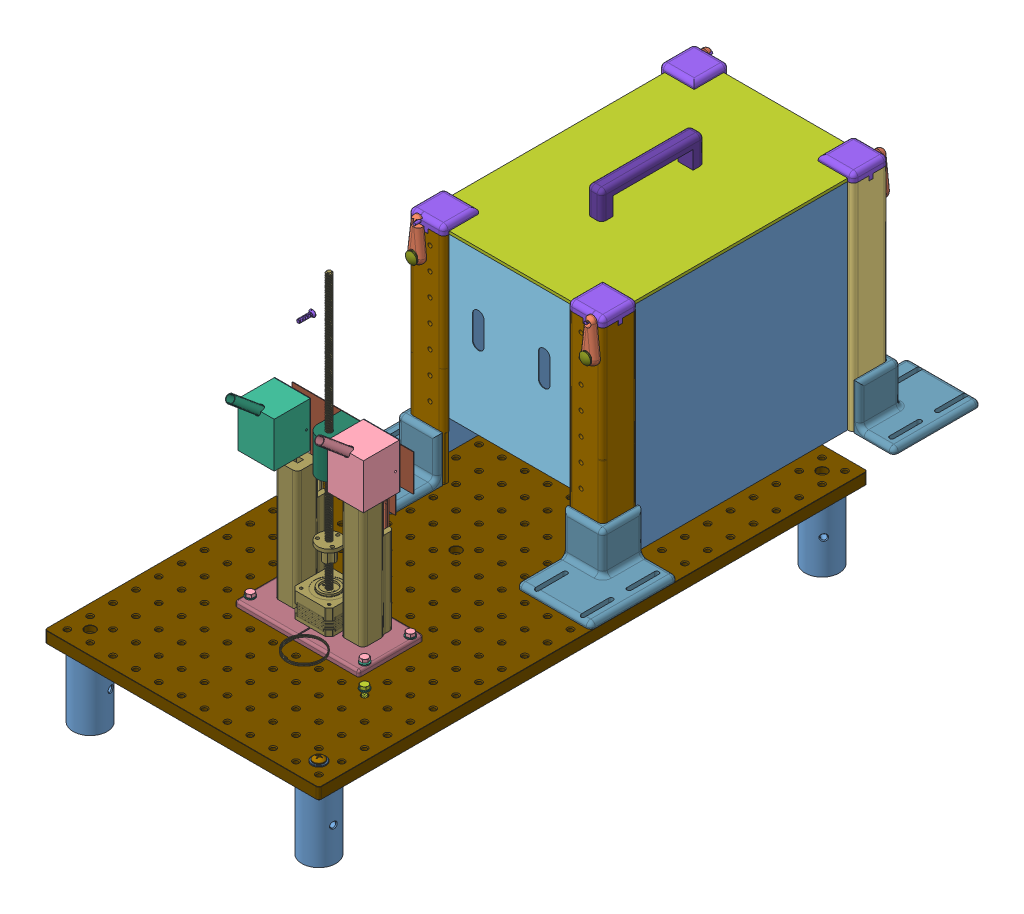
SolidWorks assembly Cage_model, configuration Default. Lengths in mm.
Overall size (306.09 428.48 734.93).
48 component instances, 32 part files, 99 mates.
Components (placement in the parent):
- Cage_acryllic_main-1: Cage_acryllic_main [Default] at (116.4275 -22.4186 -670.5141) size (203.2 239 304.17)
- Locking Mechanism^Cage_model-1: Locking Mechanism^Cage_model [Default] at (119.1314 -13.6836 -620.5993) x (0.989545 0 -0.144222) z (0.144222 0 0.989545) size (209.18 47.14 36.28) (virtual)
- Rear Legs^Cage_model-1: Rear Legs^Cage_model [Default] at (116.4275 -20.4186 -670.5141) x (0 0 -1) z (1 0 0) size (39.08 239 215.9) (virtual)
- Copy of Copy of Tube_Housing^Cage_model-1: Copy of Copy of Tube_Housing^Cage_model [Default] at (-6024.2431 5876.1322 -191.2968) size (40 77.55 71.62) (virtual)
- Stainless_steel_faceplate^Cage_model-1: Stainless_steel_faceplate^Cage_model [Default] at (116.4275 -20.4186 -366.3391) x (1 0 0) z (0 0 -1) size (203.2 177 12.61)
- Copy of Tube_Housing^Cage_model-2: Copy of Tube_Housing^Cage_model [Default] at (-6110.9268 5878.9507 -178.946) size (40 77.55 71.62) (virtual)
- cage top^Cage_model-1: cage top^Cage_model [Default] at (115.7745 -70.1218 -667.66) size (203.2 3.18 304.78) (virtual)
- Top Securing Mechanisms-1: Top Securing Mechanisms [Default] at (-397.5627 136.2654 -798.1889) x (0 0 -1) z (0 1 0) size (45.43 215.9 14.36)
- doorMotorStand ^Cage_model-1: doorMotorStand ^Cage_model [Default] at (-254.8675 208.1203 679.8373) x (1 0 0) z (0 1 0) (virtual)
- Front legs^Cage_model-2: Front legs^Cage_model [Default] at (-86.7725 -20.4186 -365.7295) x (0 0 1) z (-1 0 0) size (39.36 239 215.9) (virtual)
- Locking Mechanism^Cage_model-2: Locking Mechanism^Cage_model [Default] at (-90.3528 -13.1056 -415.6444) x (-0.989536 0.004347 0.144222) z (-0.144221 0.000634 -0.989545) size (209.18 47.14 36.28) (virtual)
- Top Securing Mechanisms-3: Top Securing Mechanisms [Default] at (427.2177 136.2654 -238.0548) x (0 0 1) z (0 1 0) size (45.43 215.9 14.36)
- Housing Door^Cage_model-1: Housing Door^Cage_model [Default] at (-6024.2431 5876.1322 -183.7968) x (-1 0 0) z (0 0 -1) size (40 50 0.61) (virtual)
- Door-2: Door [Default] at (467.6811 -160.8236 14.8493) x (0.996569 0.000281 -0.082761) z (-0.082738 -0.020299 -0.996365) size (134.22 71.08 12.57)
- Part6^Cage_model-4: Part6^Cage_model [Default] at (95.2928 -92.5203 546.9194) size (25.4 134.62 36.77) (virtual)
- Mounting Bracket nozzle holder-1: Mounting Bracket nozzle holder [Default] at (14.5275 -22.4186 -254) x (0 0 1) z (0 1 0) size (71.72 137.74 6.35)
- Angle Bracket_Leg Securing Mechanism-1: Angle Bracket_Leg Securing Mechanism [Default] at (156.2683 -22.4186 -123.1441) x (1 0 0) z (0 1 0) size (304.2 433 50.8)
- Part6^Cage_model-5: Part6^Cage_model [Default] at (168.4928 -92.5203 546.8933) size (25.4 134.62 36.77) (virtual)
- Housing Door^Cage_model-2: Housing Door^Cage_model [Default] at (-6110.9268 5878.9507 -171.446) x (-1 0 0) z (0 0 -1) size (40 50 0.61) (virtual)
- Linear Motion Attachment Housing -2: Linear Motion Attachment Housing  [Default] at (68.2215 2233.7833 0) size (25.4 40.64 38.78)
- Part9^Cage_model-2: Part9^Cage_model [Default] at (239.0332 27.7971 -363.0295) x (0.96536 0.260922 0) z (0 0 1) size (12.58 12.58 14.5) (virtual)
- Part9^Cage_model-1: Part9^Cage_model [Default] at (-93.8399 -16.6938 -363.0295) x (0.891037 -0.453931 0) z (0 0 1) size (12.58 12.58 14.5) (virtual)
- Top Handle^Cage_model-1: Top Handle^Cage_model [Default] at (-0.1143 219.7614 49.6875) x (1 0 0) z (0 1 0) size (16.56 114.3 30) (virtual)
- locking_mechanism^Cage_model-1: locking_mechanism^Cage_model [Default] at (0 0 310.525) (virtual)
- MB1224-Solidworks-1: MB1224-Solidworks [Default] at (14.5275 -35.1186 -304.8) x (0 0 1) z (-1 0 0) size (609.6 12.7 304.8)
- P3-Solidworks-1: P3-Solidworks [Web Part] at (-112.4725 -73.2186 -25.4) x (0.255609 0 0.96678) z (-0.96678 0 0.255609) size (37.74 76.2 37.94)
- P3-Solidworks-2: P3-Solidworks [Web Part] at (141.5275 -73.2186 -25.4) x (0.123275 0 -0.992373) z (0.992373 0 0.123275) size (37.74 76.2 37.94)
- P3-Solidworks-3: P3-Solidworks [Web Part] at (141.5275 -73.2186 -584.2) x (0.652104 0 -0.75813) z (0.75813 0 0.652104) size (37.74 76.2 37.94)
- P3-Solidworks-4: P3-Solidworks [Web Part] at (-112.4725 -73.2186 -584.2) x (-0.90982 0 0.415002) z (-0.415002 0 -0.90982) size (37.74 76.2 37.94)
- 3363N14_Miniature Pass-Through Drawer Slides-1: 3363N14_Miniature Pass-Through Drawer Slides [3363N14] at (51.1275 42.2414 -183.1224) x (0 1 0) z (0 0 -1) size (99.77 16 6)
- 3363N14_Miniature Pass-Through Drawer Slides (1)-1: 3363N14_Miniature Pass-Through Drawer Slides (1) [3363N14] at (-22.0725 42.2414 -183.0962) x (0 1 0) z (0 0 -1) size (99.77 16 6)
- 91287A126_18-8 Stainless Steel Hex Head Screw (1)-1: 91287A126_18-8 Stainless Steel Hex Head Screw (1) [91287A126] at (78.0275 -24.6886 -139.7) x (0.924716 0 -0.380657) z (0 1 0) size (8 9.24 28.87)
- 91028A658_JIS Hex Nut-1: 91028A658_JIS Hex Nut [91028A658] at (78.0275 -37.1186 -139.7) x (-0.777282 0 -0.629153) z (0.629153 0 -0.777282) size (8 4.57 9.24)
- 93475A240_18-8 Stainless Steel Washer-4: 93475A240_18-8 Stainless Steel Washer [93475A240] at (-48.9725 -16.0686 -190.5) x (-0.837169 0 -0.546944) z (0 1 0) size (10 10 1.1)
- 93475A240_18-8 Stainless Steel Washer-5: 93475A240_18-8 Stainless Steel Washer [93475A240] at (-48.9725 -14.9686 -139.7) x (1 0 0) z (0 -1 0) size (10 10 1.1)
- 93475A240_18-8 Stainless Steel Washer-8: 93475A240_18-8 Stainless Steel Washer [93475A240] at (78.0275 -14.9686 -190.5) x (1 0 0) z (0 -1 0) size (10 10 1.1)
- 93475A240_18-8 Stainless Steel Washer-9: 93475A240_18-8 Stainless Steel Washer [93475A240] at (78.0275 -16.0686 -139.7) x (0.591262 0 -0.806479) z (0 1 0) size (10 10 1.1)
- 91287A126_18-8 Stainless Steel Hex Head Screw (1)-5: 91287A126_18-8 Stainless Steel Hex Head Screw (1) [91287A126] at (-48.9725 -25.7186 -139.7) x (0.441314 0 0.897353) z (0 1 0) size (8 9.24 28.87)
- 91287A126_18-8 Stainless Steel Hex Head Screw (1)-6: 91287A126_18-8 Stainless Steel Hex Head Screw (1) [91287A126] at (-48.9725 -25.7186 -190.5) x (0.441314 0 0.897353) z (0 1 0) size (8 9.24 28.87)
- 91287A126_18-8 Stainless Steel Hex Head Screw (1)-9: 91287A126_18-8 Stainless Steel Hex Head Screw (1) [91287A126] at (78.0275 -25.7186 -190.5) x (0.293454 0 0.955973) z (0 1 0) size (8 9.24 28.87)
- 91287A127_18-8 Stainless Steel Hex Head Screw-1: 91287A127_18-8 Stainless Steel Hex Head Screw [91287A127] at (103.4275 -28.2186 -114.3) x (-0.998064 0 -0.062199) z (0 1 0) size (8 9.24 33.9)
- 93475A240_18-8 Stainless Steel Washer-10: 93475A240_18-8 Stainless Steel Washer [93475A240] at (103.4275 -16.0686 -114.3) x (-0.837169 0 -0.546944) z (0 1 0) size (10 10 1.1)
- 91028A658_JIS Hex Nut-4: 91028A658_JIS Hex Nut [91028A658] at (103.4275 -37.1186 -114.3) x (-0.799453 0 0.600729) z (-0.600729 0 -0.799453) size (8 4.57 9.24)
- 91430A226_18-8 Stainless Steel Slotted Flat Head Screws-1: 91430A226_18-8 Stainless Steel Slotted Flat Head Screws [91430A226] at (-69.0425 201.5814 -220.8715) x (0 0 1) z (0.071343 -0.997452 0) size (16.28 7.5 7.43)
- 91772A541_Passivated 18-8 Stainless Steel Pan Head Phillips Screw (1)-1: 91772A541_Passivated 18-8 Stainless Steel Pan Head Phillips Screw (1) [91772A541] at (141.5275 -30.2609 -25.4) x (-0.969827 0 0.243795) z (0 1 0) size (12.5 12.5 27.18)
- 90107A029_316 Stainless Steel Washer-1: 90107A029_316 Stainless Steel Washer [90107A029] at (141.5275 -21.7836 -25.4) x (0.985495 0 0.169704) z (0 1 0) size (15.88 15.88 1.27)
- LA1700-Solidworks-1: LA1700-Solidworks [Default] at (68.1361 144.7902 -179.561) x (0 -0.690695 0.723146) z (-1 0 0) size (6 6 1.79)
- 8677N21_Stepper Motor with Linear Actuation-1: 8677N21_Stepper Motor with Linear Actuation [8677N21] at (14.5275 163.7634 -163.8403) x (0 -1 0) z (1 0 0) size (339.67 87.09 59.64)
Mates (geometry in assembly coordinates):
- Front right post alignment to breadboard: coincident anti-aligned: plane of MB1224-Solidworks-1 through (-134.8725 -35.1186 -606.6) normal (0 -1 0); plane of P3-Solidworks-1 through (-112.4725 -35.1186 -25.4) normal (0 1 0)
- Rear left post hole alignement : concentric anti-aligned: circle of MB1224-Solidworks-1; circle of P3-Solidworks-3
- Rear right post hole alignment: concentric anti-aligned: circle of MB1224-Solidworks-1; circle of P3-Solidworks-4
- rear left post to breadboard: coincident anti-aligned: plane of MB1224-Solidworks-1 through (-134.8725 -35.1186 -606.6) normal (0 -1 0); plane of P3-Solidworks-3 through (141.5275 -35.1186 -584.2) normal (0 1 0)
- rear right post to breadboard: coincident anti-aligned: plane of MB1224-Solidworks-1 through (-134.8725 -35.1186 -606.6) normal (0 -1 0); plane of P3-Solidworks-4 through (-112.4725 -35.1186 -584.2) normal (0 1 0)
- Front right post hole alignment: concentric anti-aligned: circle of MB1224-Solidworks-1; circle of P3-Solidworks-1
- Coincident110: coincident anti-aligned: plane of Cage_acryllic_main-1 through (116.4275 -22.4186 -366.3391) normal (0 0 1); plane of Stainless_steel_faceplate^Cage_model-1 through (116.4275 -20.4186 -366.3391) normal (0 0 -1)
- Coincident111: coincident aligned: plane of Cage_acryllic_main-1 through (116.4275 -22.4186 -667.3391) normal (1 0 0); plane of Stainless_steel_faceplate^Cage_model-1 through (116.4275 216.5814 -365.7295) normal (1 0 0)
- Coincident112: coincident aligned: plane of Cage_acryllic_main-1 through (116.4275 216.5814 -667.3391) normal (0 1 0); plane of Stainless_steel_faceplate^Cage_model-1 through (-86.7725 216.5814 -365.7295) normal (0 1 0)
- Coincident115: coincident anti-aligned: plane of Stainless_steel_faceplate^Cage_model-1 through (116.4275 -20.4186 -365.7295) normal (0 0 1); plane of Front legs^Cage_model-2 through (-86.7725 -20.4186 -365.7295) normal (0 0 -1)
- Coincident116: coincident anti-aligned: plane of Cage_acryllic_main-1 through (116.4275 -22.4186 -667.3391) normal (1 0 0); plane of Front legs^Cage_model-2 through (116.4275 -20.4186 -365.7295) normal (-1 0 0)
- Coincident124: coincident anti-aligned: plane of Cage_acryllic_main-1 through (116.4275 -22.4186 -670.5141) normal (0 0 -1); plane of Rear Legs^Cage_model-1 through (116.4275 -20.4186 -670.5141) normal (0 0 1)
- Coincident125: coincident anti-aligned: plane of Cage_acryllic_main-1 through (116.4275 -22.4186 -667.3391) normal (1 0 0); plane of Rear Legs^Cage_model-1 through (116.4275 -20.4186 -670.5141) normal (-1 0 0)
- Coincident127: coincident anti-aligned: plane of Cage_acryllic_main-1 through (116.4275 216.5814 -667.3391) normal (0 1 0); plane of cage top^Cage_model-1 through (115.7745 216.5814 -667.66) normal (0 -1 0)
- Parallel2: parallel aligned: plane of MB1224-Solidworks-1 through (-137.8725 -22.4186 -606.6) normal (-1 0 0); plane of Front legs^Cage_model-2 through (-93.1225 -20.4186 -365.7295) normal (-1 0 0)
- Coincident130: coincident aligned: plane of Cage_acryllic_main-1 through (116.4275 -22.4186 -667.3391) normal (1 0 0); plane of cage top^Cage_model-1 through (116.4275 219.7614 -670.5141) normal (1 0 0)
- Coincident131: coincident aligned: plane of Stainless_steel_faceplate^Cage_model-1 through (116.4275 -20.4186 -365.7295) normal (0 0 1); plane of cage top^Cage_model-1 through (-86.7725 219.7614 -365.7295) normal (0 0 1)
- Coincident133: coincident aligned: plane of Rear Legs^Cage_model-1 through (122.7775 -20.4186 -670.5141) normal (1 0 0); plane of Top Securing Mechanisms-1 through (122.7775 281.3795 -798.1889) normal (1 0 0)
- Coincident134: coincident aligned: plane of Rear Legs^Cage_model-1 through (116.4275 -20.4186 -676.8641) normal (0 0 -1); plane of Top Securing Mechanisms-1 through (-397.5627 281.3795 -676.8641) normal (0 0 -1)
- Coincident136: coincident anti-aligned: plane of Front legs^Cage_model-2 through (122.7775 216.5814 -365.7295) normal (0 1 0); plane of Top Securing Mechanisms-3 through (-397.5627 216.5814 -238.0548) normal (0 -1 0)
- Coincident137: coincident aligned: plane of Front legs^Cage_model-2 through (122.7775 -20.4186 -365.7295) normal (1 0 0); plane of Top Securing Mechanisms-3 through (122.7775 281.3795 -238.0548) normal (1 0 0)
- Lock1: lock: 
- Lock2: lock: 
- Coincident234: coincident aligned: plane of MB1224-Solidworks-1 through (-134.8725 -22.4186 0) normal (0 0 1)
- Coincident253: coincident anti-aligned: plane of Copy of Tube_Housing^Cage_model-2 through (-6110.9268 5878.9507 -171.446) normal (0 0 -1); plane of Housing Door^Cage_model-2 through (-6110.9268 5878.9507 -171.446) normal (0 0 1)
- Coincident254: coincident aligned: plane of Copy of Tube_Housing^Cage_model-2 through (-54.1526 175.7249 -131.446) normal (0 1 0); plane of Housing Door^Cage_model-2 through (-14.1526 175.7249 -172.0556) normal (0 1 0)
- Coincident255: coincident aligned: plane of Copy of Tube_Housing^Cage_model-2 through (-54.1526 175.7249 -131.446) normal (-1 0 0); plane of Housing Door^Cage_model-2 through (-54.1526 175.7249 -172.0556) normal (-1 0 0)
- Coincident258: coincident anti-aligned: plane of MB1224-Solidworks-1 through (-134.8725 -22.4186 -606.6) normal (0 1 0); plane of Mounting Bracket nozzle holder^Cage_model-1 through (14.5275 -22.4186 -254) normal (0 -1 0)
- Coincident272: coincident anti-aligned: plane of Front legs^Cage_model-2 through (122.7775 -20.4186 -365.7295) normal (1 0 0); plane of Angle Bracket_Leg Securing Mechanism-1 through (122.7775 42.8936 -398.4604) normal (-1 0 0)
- Coincident273: coincident anti-aligned: plane of Front legs^Cage_model-2 through (116.4275 -20.4186 -359.3795) normal (0 0 1); plane of Angle Bracket_Leg Securing Mechanism-1 through (122.7775 52.871 -359.3795) normal (0 0 -1)
- Coincident274: coincident aligned: plane of MB1224-Solidworks-1 through (166.9275 -22.4186 -606.6) normal (1 0 0); plane of Angle Bracket_Leg Securing Mechanism-1 through (166.9275 42.8936 -398.4604) normal (1 0 0)
- Lock3: lock: 
- Parallel5: parallel aligned: plane of Part6^Cage_model-4 through (-9.3725 -53.9896 -152.1258) normal (0 0 1); plane of Part6^Cage_model-5 through (63.8275 -53.9896 -152.152) normal (0 0 1)
- Parallel6: parallel aligned: plane of MB1224-Solidworks-1 through (-134.8725 -22.4186 -606.6) normal (0 1 0)
- Parallel9: parallel aligned: plane of Stainless_steel_faceplate^Cage_model-1 through (-86.7725 216.5814 -365.7295) normal (0 1 0); plane of 3363N14_Miniature Pass-Through Drawer Slides-1 through (55.7775 107.007 -185.6224) normal (0 1 0)
- Concentric58: concentric aligned: cylinder of Mounting Bracket nozzle holder^Cage_model-1 through (78.0275 -8.8485 -139.7) axis (0 -1 0) radius 2.5527; cone of 91287A126_18-8 Stainless Steel Hex Head Screw (1)-1 through (78.0275 -13.9386 -139.7) axis (0 -1 0)
- Screw1: screw = 1 anti-aligned: cone of 91287A126_18-8 Stainless Steel Hex Head Screw (1)-1 through (78.0275 -38.9386 -139.7) axis (0 -1 0); cone of 91028A658_JIS Hex Nut-1 through (78.0275 -39.1186 -139.7) axis (0 1 0)
- Coincident295: coincident anti-aligned: plane of MB1224-Solidworks-1 through (-134.8725 -35.1186 -606.6) normal (0 -1 0); plane of 91028A658_JIS Hex Nut-1 through (78.0275 -35.1186 -139.7) normal (0 1 0)
- Coincident311: coincident aligned: plane of 3363N14_Miniature Pass-Through Drawer Slides-1 through (55.7775 107.007 -185.6224) normal (0 1 0); plane of 3363N14_Miniature Pass-Through Drawer Slides (1)-1 through (-17.4225 107.007 -185.5962) normal (0 1 0)
- Coincident312: coincident anti-aligned: plane of Part6^Cage_model-5 through (61.7475 7.2414 -210.1867) normal (0 1 0); plane of 3363N14_Miniature Pass-Through Drawer Slides-1 through (59.1275 7.2414 -188.1224) normal (0 -1 0)
- Coincident313: coincident anti-aligned: plane of Part6^Cage_model-5 through (59.1275 -40.1591 -183.1224) normal (-1 0 0); plane of 3363N14_Miniature Pass-Through Drawer Slides-1 through (59.1275 7.2414 -188.1224) normal (1 0 0)
- Coincident320: coincident anti-aligned: plane of Mounting Bracket nozzle holder^Cage_model-1 through (14.5275 -16.0686 -254) normal (0 1 0); plane of 93475A240_18-8 Stainless Steel Washer-5 through (-48.9725 -16.0686 -139.7) normal (0 -1 0)
- Concentric68: concentric anti-aligned: cylinder of Mounting Bracket nozzle holder^Cage_model-1 through (-48.9725 -8.8485 -139.7) axis (0 -1 0) radius 2.5527; cylinder of 93475A240_18-8 Stainless Steel Washer-5 through (-48.9725 -16.0686 -139.7) axis (0 1 0) radius 2.65
- Coincident321: coincident anti-aligned: plane of Mounting Bracket nozzle holder^Cage_model-1 through (14.5275 -16.0686 -254) normal (0 1 0); plane of 93475A240_18-8 Stainless Steel Washer-4 through (-48.9725 -16.0686 -190.5) normal (0 -1 0)
- Concentric69: concentric aligned: cylinder of Mounting Bracket nozzle holder^Cage_model-1 through (-48.9725 -8.8485 -190.5) axis (0 -1 0) radius 2.5527; cylinder of 93475A240_18-8 Stainless Steel Washer-4 through (-48.9725 -14.9686 -190.5) axis (0 -1 0) radius 2.65
- Coincident3241: coincident anti-aligned: plane of Mounting Bracket nozzle holder^Cage_model-1 through (14.5275 -16.0686 -254) normal (0 1 0); plane of 93475A240_18-8 Stainless Steel Washer-8 through (78.0275 -16.0686 -190.5) normal (0 -1 0)
- Concentric72: concentric anti-aligned: cylinder of Mounting Bracket nozzle holder^Cage_model-1 through (78.0275 -8.8485 -190.5) axis (0 -1 0) radius 2.5527; cylinder of 93475A240_18-8 Stainless Steel Washer-8 through (78.0275 -16.0686 -190.5) axis (0 1 0) radius 2.65
- Coincident3251: coincident anti-aligned: plane of Mounting Bracket nozzle holder^Cage_model-1 through (14.5275 -16.0686 -254) normal (0 1 0); plane of 93475A240_18-8 Stainless Steel Washer-9 through (78.0275 -16.0686 -139.7) normal (0 -1 0)
- Concentric73: concentric aligned: circle of Mounting Bracket nozzle holder^Cage_model-1; cylinder of 93475A240_18-8 Stainless Steel Washer-9 through (78.0275 -14.9686 -139.7) axis (0 -1 0) radius 2.65
- Concentric75: concentric aligned: cylinder of Mounting Bracket nozzle holder^Cage_model-1 through (-48.9725 -8.8485 -139.7) axis (0 -1 0) radius 2.5527; cone of 91287A126_18-8 Stainless Steel Hex Head Screw (1)-5 through (-48.9725 -14.9686 -139.7) axis (0 -1 0)
- Coincident329: coincident anti-aligned: plane of 93475A240_18-8 Stainless Steel Washer-5 through (-48.9725 -14.9686 -139.7) normal (0 1 0); plane of 91287A126_18-8 Stainless Steel Hex Head Screw (1)-5 through (-44.8278 -14.9686 -141.7383) normal (0 -1 0)
- Concentric76: concentric aligned: cylinder of Mounting Bracket nozzle holder^Cage_model-1 through (-48.9725 -8.8485 -190.5) axis (0 -1 0) radius 2.5527; cone of 91287A126_18-8 Stainless Steel Hex Head Screw (1)-6 through (-48.9725 -14.9686 -190.5) axis (0 -1 0)
- Coincident330: coincident anti-aligned: plane of 93475A240_18-8 Stainless Steel Washer-4 through (-48.9725 -14.9686 -190.5) normal (0 1 0); plane of 91287A126_18-8 Stainless Steel Hex Head Screw (1)-6 through (-44.8278 -14.9686 -192.5383) normal (0 -1 0)
- Concentric79: concentric aligned: cylinder of Mounting Bracket nozzle holder^Cage_model-1 through (78.0275 -8.8485 -190.5) axis (0 -1 0) radius 2.5527; cone of 91287A126_18-8 Stainless Steel Hex Head Screw (1)-9 through (78.0275 -14.9686 -190.5) axis (0 -1 0)
- Coincident333: coincident anti-aligned: plane of 93475A240_18-8 Stainless Steel Washer-8 through (78.0275 -14.9686 -190.5) normal (0 1 0); plane of 91287A126_18-8 Stainless Steel Hex Head Screw (1)-9 through (82.443 -14.9686 -191.8554) normal (0 -1 0)
- Coincident3252: coincident aligned: plane of Front legs^Cage_model-2 through (116.4275 -20.4186 -359.3795) normal (0 0 1); plane of Top Securing Mechanisms-3 through (-397.5627 281.3795 -359.3795) normal (0 0 1)
- Coincident3255: coincident anti-aligned: plane of Angle Bracket_Leg Securing Mechanism-1 through (14.8275 -16.0686 -427.9441) normal (0 1 0); plane of 93475A240_18-8 Stainless Steel Washer-10 through (103.4275 -16.0686 -114.3) normal (0 -1 0)
- Concentric657: concentric anti-aligned: cylinder of MB1224-Solidworks-1 through (103.4275 -22.4186 -114.3) axis (0 1 0) radius 2.5527; cylinder of 93475A240_18-8 Stainless Steel Washer-10 through (103.4275 -14.9686 -114.3) axis (0 -1 0) radius 2.65
- Coincident3256: coincident anti-aligned: plane of 91287A127_18-8 Stainless Steel Hex Head Screw-1 through (103.1402 -14.9686 -109.6901) normal (0 -1 0); plane of 93475A240_18-8 Stainless Steel Washer-10 through (103.4275 -14.9686 -114.3) normal (0 1 0)
- Concentric658: concentric aligned: cone of 91287A127_18-8 Stainless Steel Hex Head Screw-1 through (103.4275 -44.9686 -114.3) axis (0 -1 0); cylinder of 93475A240_18-8 Stainless Steel Washer-10 through (103.4275 -14.9686 -114.3) axis (0 -1 0) radius 2.65
- Screw4: screw = 1 aligned: cone of 91287A127_18-8 Stainless Steel Hex Head Screw-1 through (103.4275 -44.9686 -114.3) axis (0 -1 0); cone of 91028A658_JIS Hex Nut-4 through (103.4275 -35.1186 -114.3) axis (0 -1 0)
- Coincident3257: coincident anti-aligned: plane of MB1224-Solidworks-1 through (-134.8725 -35.1186 -606.6) normal (0 -1 0); plane of 91028A658_JIS Hex Nut-4 through (103.4275 -35.1186 -114.3) normal (0 1 0)
- Concentric668: concentric anti-aligned: circle of MB1224-Solidworks-1; circle of P3-Solidworks-2
- Concentric672: concentric anti-aligned: cylinder of MB1224-Solidworks-1 through (141.5275 -22.4186 -25.4) axis (0 1 0) radius 3.3; cone of 91772A541_Passivated 18-8 Stainless Steel Pan Head Phillips Screw (1)-1 through (141.5275 -43.5959 -25.4) axis (0 -1 0)
- Concentric673: concentric anti-aligned: cylinder of P3-Solidworks-2 through (141.5275 -35.3726 -25.4) axis (0 1 0) radius 3.175; cone of 91772A541_Passivated 18-8 Stainless Steel Pan Head Phillips Screw (1)-1 through (141.5275 -43.5959 -25.4) axis (0 -1 0)
- Concentric674: concentric aligned: cone of 91772A541_Passivated 18-8 Stainless Steel Pan Head Phillips Screw (1)-1 through (141.5275 -43.5959 -25.4) axis (0 -1 0); cylinder of 90107A029_316 Stainless Steel Washer-1 through (141.5275 -21.1486 -25.4) axis (0 -1 0) radius 3.5687
- Coincident3266: coincident anti-aligned: plane of MB1224-Solidworks-1 through (-134.8725 -22.4186 -606.6) normal (0 1 0); plane of 90107A029_316 Stainless Steel Washer-1 through (141.5275 -22.4186 -25.4) normal (0 -1 0)
- Tangent2: tangent anti-aligned: torus of 91772A541_Passivated 18-8 Stainless Steel Pan Head Phillips Screw (1)-1; plane of 90107A029_316 Stainless Steel Washer-1 through (141.5275 -21.1486 -25.4) normal (0 1 0)
- Screw8: screw = 1 anti-aligned: cylinder of P3-Solidworks-2 through (141.5275 -35.3726 -25.4) axis (0 1 0) radius 3.175; cone of 91772A541_Passivated 18-8 Stainless Steel Pan Head Phillips Screw (1)-1 through (141.5275 -43.5959 -25.4) axis (0 -1 0)
- Coincident3267: coincident anti-aligned: plane of MB1224-Solidworks-1 through (-134.8725 -35.1186 -606.6) normal (0 -1 0); plane of P3-Solidworks-2 through (141.5275 -35.1186 -25.4) normal (0 1 0)
- Lock7: lock: 
- Lock8: lock: 
- Coincident3292: coincident aligned: plane of Cage_acryllic_main-1 through (116.4275 216.5814 -667.3391) normal (0 1 0); plane of Front legs^Cage_model-2 through (-93.1225 216.5814 -365.7295) normal (0 1 0)
- Coincident3293: coincident aligned: plane of Front legs^Cage_model-2 through (83.6975 -22.4186 -404.8607) normal (0 -1 0); plane of Angle Bracket_Leg Securing Mechanism-1 through (156.2683 -22.4186 -123.1441) normal (0 -1 0)
- Coincident3297: coincident anti-aligned: plane of Angle Bracket_Leg Securing Mechanism-1 through (-126.6133 -22.4186 -123.1441) normal (0 -1 0); plane of MB1224-Solidworks-1 through (-134.8725 -22.4186 -606.6) normal (0 1 0)
- Concentric681: concentric anti-aligned: circle of Front legs^Cage_model-2; cylinder of Part9^Cage_model-2 through (111.3475 187.1174 -338.8874) axis (0 0 -1) radius 5
- Tangent3: tangent anti-aligned: plane of Locking Mechanism^Cage_model-2 through (111.3513 186.8113 -353.0295) normal (0 0 1); torus of Part9^Cage_model-2
- Concentric682: concentric anti-aligned: circle of Front legs^Cage_model-2; cylinder of Part9^Cage_model-1 through (-81.6925 187.1174 -338.8874) axis (0 0 -1) radius 5
- Tangent4: tangent anti-aligned: plane of Locking Mechanism^Cage_model-2 through (-81.6869 187.6593 -353.0295) normal (0 0 1); torus of Part9^Cage_model-1
- Coincident3305: coincident aligned: plane of Door-2 through (-32.6925 122.3934 -189.9191) normal (-1 0 0); plane of Part6^Cage_model-4 through (-32.6925 7.2414 -210.1605) normal (-1 0 0)
- Coincident3308: coincident aligned: plane of Door-2 through (-52.6315 163.0334 -189.9191) normal (0 1 0); plane of Part8^Cage_model-2 through (14.5275 163.0334 -163.8403) normal (0 1 0)
- Coincident3309: coincident anti-aligned: plane of MB1224-Solidworks-1 through (-134.8725 -22.4186 -606.6) normal (0 1 0); plane of 8677N21_Stepper Motor with Linear Actuation-1 through (14.5275 -22.4186 -163.8403) normal (0 -1 0)
- Coincident3313: coincident anti-aligned: plane of Mounting Bracket nozzle holder^Cage_model-1 through (-6.5672 -22.4186 -184.935) normal (1 0 0); plane of 8677N21_Stepper Motor with Linear Actuation-1 through (-6.5672 11.3634 -163.8403) normal (-1 0 0)
- Coincident3314: coincident anti-aligned: plane of Mounting Bracket nozzle holder^Cage_model-1 through (35.6222 -22.4186 -184.935) normal (0 0 1); plane of 8677N21_Stepper Motor with Linear Actuation-1 through (14.5275 11.3634 -184.935) normal (0 0 -1)
- Concentric685: concentric aligned: cylinder of Part8^Cage_model-2 through (14.5275 112.4939 -163.8403) axis (0 1 0) radius 3.5; cone of 8677N21_Stepper Motor with Linear Actuation-1 through (14.5275 314.9728 -163.8403) axis (0 1 0)
- Concentric686: concentric anti-aligned: cylinder of Part8^Cage_model-2 through (22.7764 128.3934 -159.0778) axis (0 -1 0) radius 1.778; circle of 8677N21_Stepper Motor with Linear Actuation-1
- Concentric689: concentric aligned: circle of Stainless_steel_faceplate^Cage_model-1; circle of 91430A226_18-8 Stainless Steel Slotted Flat Head Screws-1
- Coincident3317: coincident anti-aligned: plane of Door-2 through (467.6811 -160.8236 -189.9191) normal (0 0 1); plane of Part8^Cage_model-2 through (467.6811 568.902 -189.9191) normal (0 0 -1)
- Coincident3318: coincident anti-aligned: plane of Part6^Cage_model-4 through (-30.0725 -40.1591 -183.0962) normal (0 0 -1); plane of 3363N14_Miniature Pass-Through Drawer Slides (1)-1 through (-30.0725 7.2414 -183.0962) normal (0 0 1)
- Coincident3319: coincident anti-aligned: plane of Part6^Cage_model-4 through (-30.0725 -40.1591 -183.0962) normal (1 0 0); plane of 3363N14_Miniature Pass-Through Drawer Slides (1)-1 through (-30.0725 7.2414 -188.0962) normal (-1 0 0)
- Coincident3320: coincident anti-aligned: plane of Part6^Cage_model-5 through (43.1275 -40.1591 -183.1224) normal (0 0 -1); plane of 3363N14_Miniature Pass-Through Drawer Slides-1 through (43.1275 7.2414 -183.1224) normal (0 0 1)
- Concentric692: concentric anti-aligned: circle of Copy of Tube_Housing^Cage_model-1; circle of LA1700-Solidworks-1
- Coincident3321: coincident anti-aligned: plane of Copy of Copy of Tube_Housing^Cage_model-1 through (-6024.2431 5876.1322 -183.7968) normal (0 0 -1); plane of Housing Door^Cage_model-1 through (-6024.2431 5876.1322 -183.7968) normal (0 0 1)
- Coincident3322: coincident aligned: plane of Copy of Copy of Tube_Housing^Cage_model-1 through (72.5311 172.9064 -143.7968) normal (1 0 0); plane of Housing Door^Cage_model-1 through (72.5311 172.9064 -184.4064) normal (1 0 0)
- Coincident3323: coincident aligned: plane of Copy of Copy of Tube_Housing^Cage_model-1 through (32.5311 172.9064 -143.7968) normal (0 1 0); plane of Housing Door^Cage_model-1 through (72.5311 172.9064 -184.4064) normal (0 1 0)
- Coincident3327: coincident aligned: plane of Copy of Copy of Tube_Housing^Cage_model-1 through (69.0311 144.7902 -179.561) normal (-1 0 0); circle of LA1700-Solidworks-1
- Coincident3328: coincident: point of Cage_acryllic_main-1; plane of Rear Legs^Cage_model-1 through (122.7775 216.5814 -670.5141) normal (0 1 0)
- Coincident3329: coincident anti-aligned: plane of cage top^Cage_model-1 through (115.7745 219.7614 -667.66) normal (0 1 0); plane of Top Handle^Cage_model-1 through (-0.1143 219.7614 49.6875) normal (0 -1 0)
- Lock10: lock: 
